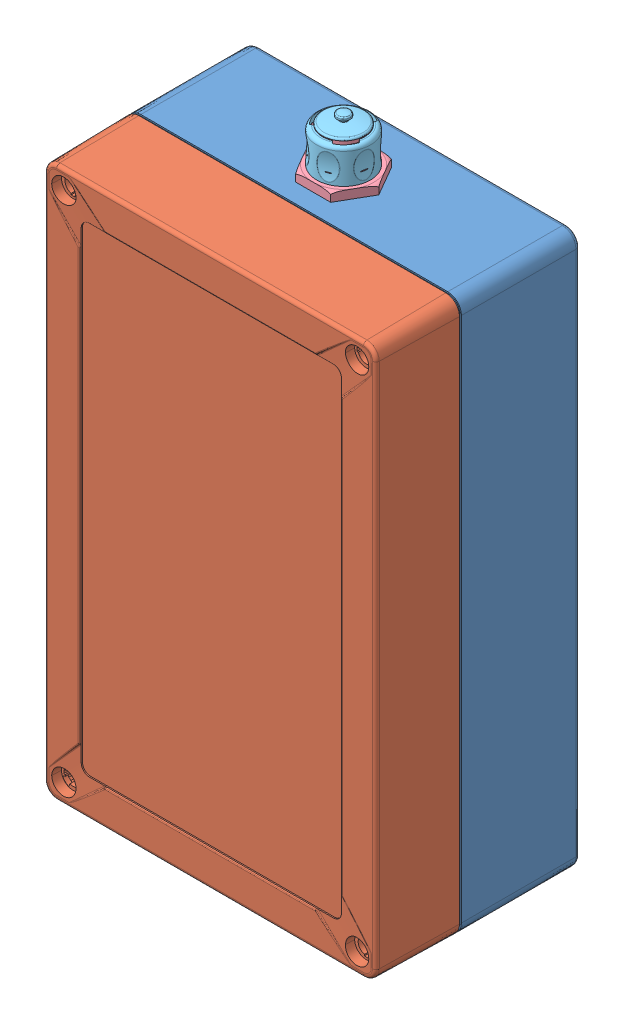
SolidWorks assembly CP_Datalogger, configuration Predeterminado. Lengths in mm.
Overall size (122 222.01 75.15).
10 component instances, 7 part files, 23 mates.
Components (placement in the parent):
- SG-22 Base-1: SG-22 Base [Predeterminado] at (-4.1607 -7.1967 22) size (122 202 46)
- SG-22 Tapa-1: SG-22 Tapa [Predeterminado] at (-4.1607 -7.1967 -43.35) size (122 202 37.76)
- SpacerWurth970300324.stp-1: SpacerWurth970300324.stp [Predeterminado] at (29.9343 -87.5527 3.4115) x (-0.84273 0.538337 0) z (0 0 1) size (6.36 6.36 30)
- SpacerWurth970300324.stp-2: SpacerWurth970300324.stp [Predeterminado] at (29.6763 72.9963 3.4115) size (6.36 6.36 30)
- SpacerWurth970300324.stp-3: SpacerWurth970300324.stp [Predeterminado] at (-38.0687 -87.5757 3.4115) size (6.36 6.36 30)
- SpacerWurth970300324.stp-4: SpacerWurth970300324.stp [Predeterminado] at (-38.2187 73.1013 3.4115) size (6.36 6.36 30)
- pxp4043-b-1: pxp4043-b [Default] at (-4.1607 110.1033 3.3) x (0 0 1) z (0 1 0) size (25.68 25.68 24.8)
- Bulgin-pxp4083-1: Bulgin-pxp4083 [Default] at (-4.1607 108.3783 3.3) x (0.465806 0 -0.884887) z (0 1 0) size (20.52 20.78 16.89)
- PowerBoard-1: PowerBoard [Predeterminado] at (-63.3357 -103.6267 -11.5885) size (112.88 192.86 37.66)
- LoggerBoard-1: LoggerBoard [Predeterminado] at (-63.3357 -103.6267 18.823) size (112.88 192.86 0.41)
Mates (geometry in assembly coordinates):
- Concéntrica8: concentric aligned: cylinder of SG-22 Base-1 through (49.3393 -100.6967 3.9) axis (0 0 -1) radius 1.6325; cone of SG-22 Tapa-1 through (49.3393 -100.6967 52) axis (0 0 -1)
- Paralelo5: parallel aligned: line of SG-22 Base-1 through (56.8393 -103.1967 21.3) axis (0 1 0); line of SG-22 Tapa-1 through (56.8393 -103.1967 22) axis (0 1 0)
- Distancia límite2: limit distance = 0 mm anti-aligned: plane of SG-22 Tapa-1 through (-4.1607 -7.1967 22) normal (0 0 -1); plane of SG-22 Base-1 through (-4.1607 -7.1967 22) normal (0 0 1)
- Concéntrica20: concentric aligned: circle of SG-22 Base-1; circle of pxp4043-b-1
- Paralelo10: parallel aligned: line of SG-22 Base-1 through (51.8393 93.8033 21.3) axis (-1 0 0); line of pxp4043-b-1 through (-1.3607 108.0857 4.5661) axis (-1 0 0)
- Coincidente16: coincident anti-aligned: plane of SG-22 Base-1 through (51.8393 93.8033 -20.5) normal (0 1 0); plane of pxp4043-b-1 through (-4.1607 93.8033 3.3) normal (0 -1 0)
- Paralelo11: parallel anti-aligned: plane of SG-22 Base-1 through (51.8393 93.8033 -20.5) normal (0 1 0); plane of Bulgin-pxp4083-1 through (-4.1607 96.9783 3.3) normal (0 -1 0)
- Concéntrica21: concentric anti-aligned: circle of pxp4043-b-1; circle of Bulgin-pxp4083-1
- Distancia límite6: limit distance = 0 mm anti-aligned: plane of Bulgin-pxp4083-1 through (-4.1607 96.9783 3.3) normal (0 -1 0); plane of pxp4043-b-1 through (-4.1607 96.9783 3.3) normal (0 1 0)
- Concéntrica22: concentric anti-aligned: circle of SG-22 Base-1; circle of PowerBoard-1
- Paralelo12: parallel aligned: line of SG-22 Base-1 through (53.8393 -92.3967 23) axis (0 1 0); line of PowerBoard-1 through (52.2793 -91.0017 -11.5885) axis (0 1 0)
- Distancia límite7: limit distance = 0 mm anti-aligned: plane of PowerBoard-1 through (33.2803 -102.0267 -12) normal (0 0 -1); plane of SG-22 Base-1 through (41.0393 -64.9467 -12) normal (0 0 1)
- Concéntrica23: concentric aligned: circle of SpacerWurth970300324.stp-1; circle of PowerBoard-1
- Concéntrica24: concentric aligned: circle of SpacerWurth970300324.stp-3; circle of PowerBoard-1
- Concéntrica25: concentric aligned: circle of SpacerWurth970300324.stp-2; circle of PowerBoard-1
- Concéntrica26: concentric aligned: circle of SpacerWurth970300324.stp-4; circle of PowerBoard-1
- Coincidente19: coincident anti-aligned: plane of SpacerWurth970300324.stp-4 through (-38.2187 73.1013 -11.5885) normal (0 0 -1); plane of PowerBoard-1 through (33.2803 -102.0267 -11.5885) normal (0 0 1)
- Coincidente20: coincident anti-aligned: plane of SpacerWurth970300324.stp-2 through (29.6763 72.9963 -11.5885) normal (0 0 -1); plane of PowerBoard-1 through (33.2803 -102.0267 -11.5885) normal (0 0 1)
- Coincidente21: coincident anti-aligned: plane of SpacerWurth970300324.stp-3 through (-38.0687 -87.5757 -11.5885) normal (0 0 -1); plane of PowerBoard-1 through (33.2803 -102.0267 -11.5885) normal (0 0 1)
- Coincidente22: coincident anti-aligned: plane of SpacerWurth970300324.stp-1 through (29.9343 -87.5527 -11.5885) normal (0 0 -1); plane of PowerBoard-1 through (33.2803 -102.0267 -11.5885) normal (0 0 1)
- Concéntrica27: concentric anti-aligned: circle of SpacerWurth970300324.stp-1; circle of LoggerBoard-1
- Paralelo13: parallel aligned: line of PowerBoard-1 through (52.2793 -91.0017 -11.5885) axis (0 1 0); line of LoggerBoard-1 through (52.2793 -91.0017 18.823) axis (0 1 0)
- Distancia límite8: limit distance = 0 mm anti-aligned: plane of LoggerBoard-1 through (33.2803 -102.0267 18.4115) normal (0 0 -1); plane of SpacerWurth970300324.stp-1 through (29.9343 -87.5527 18.4115) normal (0 0 1)
